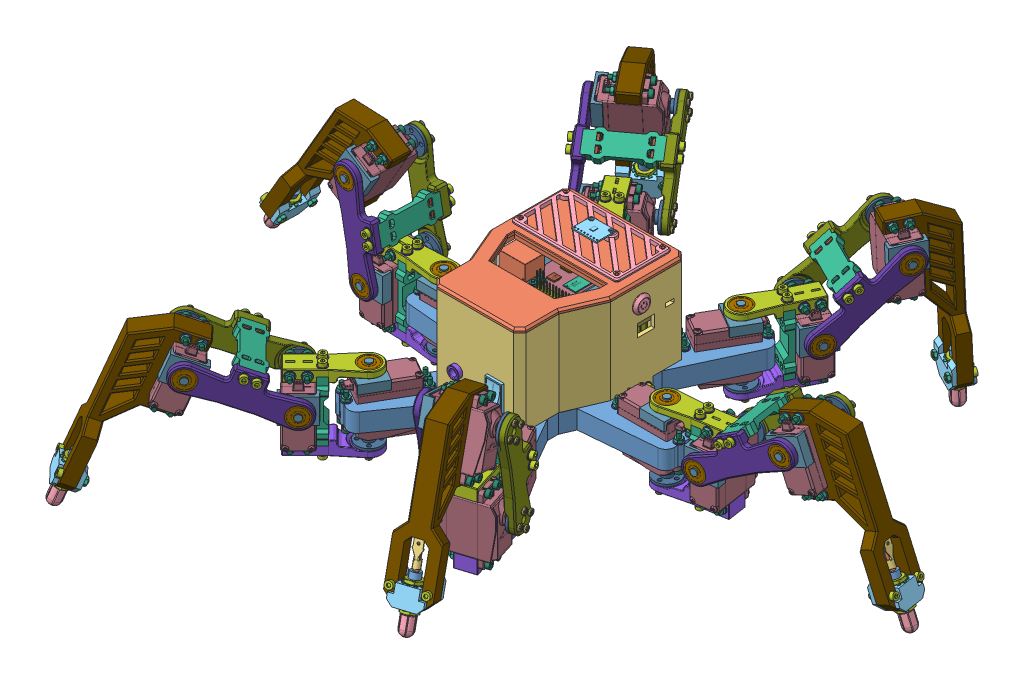
SolidWorks assembly HEXUMI_DSSERVO, configuration Default. Lengths in mm. (continued)
Components (placement in the parent): (continued)
- LEG_R-2: LEG_R [Default] at (64.2974 -8.25 149.3441) x (0.953158 0 -0.302473) z (-0.302473 0 -0.953158) size (67.5 178.11 186.84) (flexible) (continued)
  - M3_WASHER-11: M3_WASHER [Default] at (32.5 -42.9736 -1.217) x (0 0.946468 0.322799) z (0 0.322799 -0.946468) size (7 0.5 7)
  - M3_WASHER-12: M3_WASHER [Default] at (32.5 -50.8556 -2.5855) x (0 0.864489 0.502652) z (0 0.502652 -0.864489) size (7 0.5 7)
  - M3_SQUARE_NUT-10: M3_SQUARE_NUT [Default] at (-14.7 -42.9736 -1.217) x (0 -0.985259 -0.171071) z (0 -0.171071 0.985259) size (5.3 1.7 5.3)
  - M3_SQUARE_NUT-11: M3_SQUARE_NUT [Default] at (-14.7 -50.8556 -2.5855) x (0 -0.985259 -0.171071) z (0 -0.171071 0.985259) size (5.3 1.7 5.3)
  - M3_SQUARE_NUT-12: M3_SQUARE_NUT [Default] at (17.5 -42.9736 -1.217) x (0 -0.985259 -0.171071) z (0 -0.171071 0.985259) size (5.3 1.7 5.3)
  - SERVO_ASM-3: SERVO_ASM [Default] at (25.8 -78.9181 -22.175) x (0 0.943081 -0.332564) z (1 0 0) size (87.25 24.4 54.8)
    - SW2020 DS3225MG Servo 25Kg 4.8-6.8V-2: SW2020 DS3225MG Servo 25Kg 4.8-6.8V [Default] at origin size (54.3 20.4 45.91)
    - SERVO_CLIP-1: SERVO_CLIP [Default] at (0 0 -45.6) x (-1 0 0) z (0 0 -1) size (20 24.4 14.2)
  - M3_STEEL_HEX_BOLT-6: M3_STEEL_HEX_BOLT [Default] at (14.2 -94.7271 -21.9019) x (0 -0.45302 0.8915) z (0 -0.8915 -0.45302) size (5.68 28 5.68)
  - M3_STEEL_HEX_BOLT-7: M3_STEEL_HEX_BOLT [Default] at (14.2 -47.9503 -38.3971) x (0 -0.45302 0.8915) z (0 -0.8915 -0.45302) size (5.68 28 5.68)
  - M3_STEEL_HEX_BOLT-8: M3_STEEL_HEX_BOLT [Default] at (14.2 -44.6247 -28.9663) x (0 -0.45302 0.8915) z (0 -0.8915 -0.45302) size (5.68 28 5.68)
  - M3_WASHER-13: M3_WASHER [Default] at (-8.5 -91.4015 -12.4711) x (0 -0.999996 0.002865) z (0 0.002865 0.999996) size (7 0.5 7)
  - M3_WASHER-14: M3_WASHER [Default] at (-8.5 -47.9503 -38.3971) x (0 -0.195932 -0.980617) z (0 -0.980617 0.195932) size (7 0.5 7)
  - M3_WASHER-15: M3_WASHER [Default] at (-8.5 -94.7271 -21.9019) x (0 -0.288509 0.957477) z (0 0.957477 0.288509) size (7 0.5 7)
  - M3_HEX_NUT-9: M3_HEX_NUT [Default] at (-8.5 -91.4015 -12.4711) x (0 -1 -0.0006) z (0 0.0006 -1) size (6.98 2.4 5.5)
  - M3_HEX_NUT-10: M3_HEX_NUT [Default] at (-8.5 -94.7271 -21.9019) x (0 -0.879232 0.476394) z (0 -0.476394 -0.879232) size (6.98 2.4 5.5)
  - M3_HEX_NUT-11: M3_HEX_NUT [Default] at (-8.5 -44.6247 -28.9663) x (0 -0.979734 0.200301) z (0 -0.200301 -0.979734) size (6.98 2.4 5.5)
  - M3_WASHER-17: M3_WASHER [Default] at (-8.5 -44.6247 -28.9663) x (0 -0.482932 0.875658) z (0 0.875658 0.482932) size (7 0.5 7)
  - M3_SERVO_HORN_BOLT-15: M3_SERVO_HORN_BOLT [Default] at (0 28.25 30) x (0.155386 0 -0.987854) z (-0.987854 0 -0.155386) size (4.8 7 4.8)
  - M3_HEX_NUT-12: M3_HEX_NUT [Default] at (-10.9 -24.75 -5.2) x (0 -0.133559 0.991041) z (0 0.991041 0.133559) size (6.98 2.4 5.5)
  - M3_STEEL_HEX_BOLT-9: M3_STEEL_HEX_BOLT [Default] at (14.2 -24.75 -5.2) x (0 -0.73374 -0.679431) z (0 0.679431 -0.73374) size (5.68 28 5.68)
  - M3_WASHER-18: M3_WASHER [Default] at (-8.5 -24.75 -5.2) x (0 -0.999705 0.024279) z (0 0.024279 0.999705) size (7 0.5 7)
  - M3_STEEL_HEX_BOLT-10: M3_STEEL_HEX_BOLT [Default] at (14.2 -24.75 -15.2) x (0 -0.740024 -0.67258) z (0 0.67258 -0.740024) size (5.68 28 5.68)
  - M3_STEEL_HEX_BOLT-11: M3_STEEL_HEX_BOLT [Default] at (14.2 24.85 -5.2) x (0 -0.741809 -0.670611) z (0 0.670611 -0.741809) size (5.68 28 5.68)
  - M3_STEEL_HEX_BOLT-12: M3_STEEL_HEX_BOLT [Default] at (14.2 24.85 -15.2) x (0 0.582747 -0.812654) z (0 0.812654 0.582747) size (5.68 28 5.68)
  - M3_HEX_NUT-13: M3_HEX_NUT [Default] at (-10.9 24.85 -15.2) x (0 0.525669 0.850689) z (0 0.850689 -0.525669) size (6.98 2.4 5.5)
  - M3_WASHER-19: M3_WASHER [Default] at (-8.5 24.85 -15.2) x (0 -0.601111 0.799166) z (0 0.799166 0.601111) size (7 0.5 7)
  - M3_HEX_NUT-14: M3_HEX_NUT [Default] at (-10.9 24.85 -5.2) x (0 -0.636716 -0.771098) z (0 -0.771098 0.636716) size (6.98 2.4 5.5)
  - M3_WASHER-20: M3_WASHER [Default] at (-8.5 24.85 -5.2) x (0 -0.786332 -0.617804) z (0 -0.617804 0.786332) size (7 0.5 7)
  - M3_HEX_NUT-15: M3_HEX_NUT [Default] at (-10.9 -24.75 -15.2) x (0 0.444007 -0.896023) z (0 -0.896023 -0.444007) size (6.98 2.4 5.5)
  - M3_WASHER-21: M3_WASHER [Default] at (-8.5 -24.75 -15.2) x (0 -0.943365 -0.331756) z (0 -0.331756 0.943365) size (7 0.5 7)
  - TIBIA_V2_ASM-1: TIBIA_V2_ASM [Default] at (0 -78.9958 -22.0946) x (-1 0 0) z (0 -0.943081 0.332564) size (32.11 50.6 145.7)
    - TIBIA_V2-1: TIBIA_V2 [Default] at origin size (32 47.6 127.94)
    - LIMIT_SWITCH-1: LIMIT_SWITCH [Default] at (0 32.3524 -111.7407) x (-0.992713 0.1205 0) z (0.1205 0.992713 0) size (13.8 62.3 13.8) (flexible)
      - LIMIT_SWITCH_SLEEVE-1: LIMIT_SWITCH_SLEEVE [Default] at origin size (7.7 25.25 7.7)
      - LIMIT_SWITCH_SHAFT-1: LIMIT_SWITCH_SHAFT [Default] at (0 5.5422 0) x (-0.210419 0 -0.977611) z (0.977611 0 -0.210419) size (5 52 5)
      - LIMIT_SWITCH_LIMITER-1: LIMIT_SWITCH_LIMITER [Default] at (0 26.0422 0) x (-0.600712 0 -0.799465) z (0.799465 0 -0.600712) size (6.64 21.41 7.08)
      - RUBBER_CAP-1: RUBBER_CAP [Default] at (0 -9.9578 0) x (0.575853 0 -0.817553) z (0.817553 0 0.575853) size (10 14 10)
    - FOOT_HOLD-1: FOOT_HOLD [Default] at (0 32.3524 -108.9407) x (1 0 0) z (0 -1 0) size (32 22 16)
    - LIMIT_SWITCH_WASHER-1: LIMIT_SWITCH_WASHER [Default] at (0 32.3524 -93.5407) x (0.999093 -0.042592 0) z (0.042592 0.999093 0) size (14.82 0.4 15)
    - LIMIT_SWITCH_WASHER-2: LIMIT_SWITCH_WASHER [Default] at (0 32.3524 -108.9407) x (0.999093 -0.042592 0) z (0.042592 0.999093 0) size (14.82 0.4 15)
    - LIMIT_SWITCH_NUT-1: LIMIT_SWITCH_NUT [Default] at (0 32.3524 -92.3407) x (0.997292 -0.073548 0) z (0.073548 0.997292 0) size (13.86 2.4 12)
    - LIMIT_SWITCH_NUT-2: LIMIT_SWITCH_NUT [Default] at (0 32.3524 -110.5407) x (0.999648 -0.026514 0) z (0.026514 0.999648 0) size (13.86 2.4 12)
    - M3_HEX_NUT-1: M3_HEX_NUT [Default] at (-12 21.9524 -96.9407) x (-0.996596 0 -0.082443) z (0.082443 0 -0.996596) size (6.98 2.4 5.5)
    - M3_HEX_NUT-2: M3_HEX_NUT [Default] at (12 21.9524 -96.9407) x (-0.491735 0 -0.870745) z (0.870745 0 -0.491735) size (6.98 2.4 5.5)
    - M3_STEEL_HEX_BOLT_16MM-1: M3_STEEL_HEX_BOLT_16MM [Default] at (-12 40.3524 -96.9407) x (-0.809803 0 -0.586702) z (-0.586702 0 0.809803) size (5.68 19 5.68)
    - M3_STEEL_HEX_BOLT_16MM-2: M3_STEEL_HEX_BOLT_16MM [Default] at (12 40.3524 -96.9407) x (-0.933551 0 -0.358443) z (-0.358443 0 0.933551) size (5.68 19 5.68)
- LEG_R-3: LEG_R [Default] at (68.2717 -8.25 -96.793) x (-0.894785 0 -0.446496) z (-0.446496 0 0.894785) size (67.5 178.11 186.84) (flexible)
  - LINK-1: LINK [Default] at origin size (20 48.5 7)
  - COXA_BEARING-1: COXA_BEARING [Default] at (0 -29.25 30) size (20 9.2 60)
  - COXA_SERVO-1: COXA_SERVO [Default] at (0 31.25 30) x (-1 0 0) z (0 0 1) size (20 11.2 60)
  - BEARING-1: BEARING [Default] at (0 -24.25 30) x (0.102919 0 0.99469) z (0 -1 0) size (16 16 5)
  - HORN-1: HORN [Default] at (0 26.25 30) x (0 0 -1) z (0 -1 0) size (20 20 4.6)
  - M3_SQUARE_NUT-1: M3_SQUARE_NUT [Default] at (-4 16.25 3.5) x (0.944757 0 -0.327772) z (0.327772 0 0.944757) size (5.3 1.7 5.3)
  - M3_STEEL_HEX_BOLT_16MM-1: M3_STEEL_HEX_BOLT_16MM [Default] at (4 34.75 3.5) x (-0.875719 0 0.482821) z (0.482821 0 0.875719) size (5.68 19 5.68)
  - M3_WASHER-1: M3_WASHER [Default] at (4 31.25 3.5) x (0.984161 0 0.177277) z (-0.177277 0 0.984161) size (7 0.5 7)
  - M3_SERVO_HORN_BOLT-1: M3_SERVO_HORN_BOLT [Default] at (-7 33.25 30) x (-0.808099 0 -0.589047) z (-0.589047 0 0.808099) size (4.8 7 4.8)
  - M3_SERVO_HORN_BOLT-2: M3_SERVO_HORN_BOLT [Default] at (7 33.25 30) x (-0.808099 0 -0.589047) z (-0.589047 0 0.808099) size (4.8 7 4.8)
  - M3_SERVO_HORN_BOLT-3: M3_SERVO_HORN_BOLT [Default] at (0 33.25 37) x (-0.808099 0 -0.589047) z (-0.589047 0 0.808099) size (4.8 7 4.8)
  - M3_SERVO_HORN_BOLT-4: M3_SERVO_HORN_BOLT [Default] at (0 33.25 23) x (-0.808099 0 -0.589047) z (-0.589047 0 0.808099) size (4.8 7 4.8)
  - M3_SQUARE_NUT-2: M3_SQUARE_NUT [Default] at (4 16.25 3.5) x (0.947931 0 -0.318475) z (0.318475 0 0.947931) size (5.3 1.7 5.3)
  - M3_SQUARE_NUT-3: M3_SQUARE_NUT [Default] at (-4 -15.95 3.5) x (0.944757 0 -0.327772) z (0.327772 0 0.944757) size (5.3 1.7 5.3)
  - M3_SQUARE_NUT-4: M3_SQUARE_NUT [Default] at (4 -15.95 3.5) x (0.944757 0 -0.327772) z (0.327772 0 0.944757) size (5.3 1.7 5.3)
  - M3_STEEL_HEX_BOLT_16MM-2: M3_STEEL_HEX_BOLT_16MM [Default] at (-4 -32.75 3.5) x (0.944757 0 -0.327772) z (0.327772 0 0.944757) size (5.68 19 5.68)
  - M3_STEEL_HEX_BOLT_16MM-3: M3_STEEL_HEX_BOLT_16MM [Default] at (4 -32.75 3.5) x (0.944757 0 -0.327772) z (0.327772 0 0.944757) size (5.68 19 5.68)
  - M3_STEEL_HEX_BOLT_16MM-4: M3_STEEL_HEX_BOLT_16MM [Default] at (-4 34.75 3.5) x (-0.748645 0 0.662971) z (0.662971 0 0.748645) size (5.68 19 5.68)
  - M3_WASHER-2: M3_WASHER [Default] at (4 -29.75 3.5) x (0.938378 0 -0.34561) z (0.34561 0 0.938378) size (7 0.5 7)
  - M3_WASHER-3: M3_WASHER [Default] at (-4 -29.75 3.5) x (0.835901 0 -0.54888) z (0.54888 0 0.835901) size (7 0.5 7)
  - M3_WASHER-4: M3_WASHER [Default] at (-4 31.25 3.5) x (0.997383 0 -0.072301) z (0.072301 0 0.997383) size (7 0.5 7)
  - SERVO_ASM-1: SERVO_ASM [Default] at (25.8 -9.95 -10.2) x (0 1 0) z (1 0 0) size (87.25 24.4 54.8)
    - SW2020 DS3225MG Servo 25Kg 4.8-6.8V-2: SW2020 DS3225MG Servo 25Kg 4.8-6.8V [Default] at origin size (54.3 20.4 45.91)
    - SERVO_CLIP-1: SERVO_CLIP [Default] at (0 0 -45.6) x (-1 0 0) z (0 0 -1) size (20 24.4 14.2)
  - SERVO_ASM-2: SERVO_ASM [Default] at (0 24.55 30) x (0.060715 0 0.998155) z (0 1 0) size (87.25 24.4 54.8)
    - SW2020 DS3225MG Servo 25Kg 4.8-6.8V-2: SW2020 DS3225MG Servo 25Kg 4.8-6.8V [Default] at origin size (54.3 20.4 45.91)
    - SERVO_CLIP-1: SERVO_CLIP [Default] at (0 0 -45.6) x (-1 0 0) z (0 0 -1) size (20 24.4 14.2)
  - M3_SQUARE_NUT-5: M3_SQUARE_NUT [Default] at (0.85 24.85 -15.2) x (0 0 -1) z (0 1 0) size (5.3 1.7 5.3)
  - M3_SQUARE_NUT-6: M3_SQUARE_NUT [Default] at (0.85 -24.75 -5.2) x (0 1 0) z (0 0 1) size (5.3 1.7 5.3)
  - M3_SQUARE_NUT-7: M3_SQUARE_NUT [Default] at (0.85 -24.75 -15.2) x (0 1 0) z (0 0 1) size (5.3 1.7 5.3)
  - M3_SQUARE_NUT-8: M3_SQUARE_NUT [Default] at (0.85 24.85 -5.2) x (0 0 -1) z (0 1 0) size (5.3 1.7 5.3)
  - FEMUR_SERVO-1: FEMUR_SERVO [Default] at (32.5 -9.95 -10.2) x (-1 0 0) z (0 0.640618 0.76786) size (10 28 90)
  - FEMUR_BEARING-1: FEMUR_BEARING [Default] at (-28 -54.7933 -63.9502) x (1 0 0) z (0 -0.640618 -0.76786) size (8 28 90)
  - LINK-2: LINK [Default] at (1.25 -46.1931 -25.544) x (0 0.640618 0.76786) z (0 0.76786 -0.640618) size (20 48.5 7)
  - BEARING-2: BEARING [Default] at (-28 -54.7933 -63.9502) x (0 0.859543 0.511064) z (1 0 0) size (16 16 5)
  - HORN-2: HORN [Default] at (27.5 -54.7933 -63.9502) x (0 -0.76786 0.640618) z (-1 0 0) size (20 20 4.6)
  - BEARING-3: BEARING [Default] at (-28 -9.95 -10.2) x (0 0.859543 0.511064) z (1 0 0) size (16 16 5)
  - HORN-3: HORN [Default] at (27.5 -9.95 -10.2) x (0 -0.640618 -0.76786) z (-1 0 0) size (20 20 4.6)
  - M3_HEX_NUT-5: M3_HEX_NUT [Default] at (-8.5 -20.4015 -70.2245) x (0 -0.795634 0.605778) z (0 -0.605778 -0.795634) size (6.98 2.4 5.5)
  - M3_SERVO_HORN_BOLT-5: M3_SERVO_HORN_BOLT [Default] at (34.5 -60.1683 -59.4658) x (0 -0.164589 0.986362) z (0 -0.986362 -0.164589) size (4.8 7 4.8)
  - M3_SQUARE_NUT-9: M3_SQUARE_NUT [Default] at (17.5 -46.0681 -30.8576) x (0 -0.640618 -0.76786) z (0 -0.76786 0.640618) size (5.3 1.7 5.3)
  - M3_STEEL_HEX_BOLT-5: M3_STEEL_HEX_BOLT [Default] at (14.2 -69.5984 -58.3997) x (0 -0.45302 0.8915) z (0 -0.8915 -0.45302) size (5.68 28 5.68)
  - M3_STEEL_HEX_BOLT_16MM-5: M3_STEEL_HEX_BOLT_16MM [Default] at (-31.5 -46.0681 -30.8576) x (0 0.164045 0.986453) z (0 0.986453 -0.164045) size (5.68 19 5.68)
  - M3_WASHER-9: M3_WASHER [Default] at (-28.5 -46.0681 -30.8576) x (0 0.889965 0.456029) z (0 0.456029 -0.889965) size (7 0.5 7)
  - M3_SERVO_HORN_BOLT-6: M3_SERVO_HORN_BOLT [Default] at (34.5 -49.4183 -68.4345) x (0 -0.961641 0.27431) z (0 -0.27431 -0.961641) size (4.8 7 4.8)
  - M3_SERVO_HORN_BOLT-7: M3_SERVO_HORN_BOLT [Default] at (34.5 -14.4343 -15.575) x (0 -0.974393 0.224852) z (0 -0.224852 -0.974393) size (4.8 7 4.8)
  - M3_SERVO_HORN_BOLT-8: M3_SERVO_HORN_BOLT [Default] at (34.5 -4.575 -14.6843) x (0 -0.996733 0.080764) z (0 -0.080764 -0.996733) size (4.8 7 4.8)
  - M3_SERVO_HORN_BOLT-9: M3_SERVO_HORN_BOLT [Default] at (34.5 -15.325 -5.7157) x (0 -0.79921 0.601052) z (0 -0.601052 -0.79921) size (4.8 7 4.8)
  - M3_SERVO_HORN_BOLT-10: M3_SERVO_HORN_BOLT [Default] at (34.5 -5.4657 -4.825) x (0 -0.903711 0.428143) z (0 -0.428143 -0.903711) size (4.8 7 4.8)
  - M3_SERVO_HORN_BOLT-11: M3_SERVO_HORN_BOLT [Default] at (34.5 -59.2776 -69.3252) x (0 -0.961939 -0.273266) z (0 0.273266 -0.961939) size (4.8 7 4.8)
  - M3_SERVO_HORN_BOLT-12: M3_SERVO_HORN_BOLT [Default] at (34.5 -50.3089 -58.5752) x (0 -0.806511 0.591219) z (0 -0.591219 -0.806511) size (4.8 7 4.8)
  - M3_SERVO_HORN_BOLT-13: M3_SERVO_HORN_BOLT [Default] at (29.5 -9.95 -10.2) x (0 -0.903711 0.428143) z (0 -0.428143 -0.903711) size (4.8 7 4.8)
  - M3_SERVO_HORN_BOLT-14: M3_SERVO_HORN_BOLT [Default] at (29.5 -54.7933 -63.9502) x (0 -0.903711 0.428143) z (0 -0.428143 -0.903711) size (4.8 7 4.8)
  - M3_STEEL_HEX_BOLT_16MM-6: M3_STEEL_HEX_BOLT_16MM [Default] at (36 -40.9431 -24.7147) x (0 -0.934703 -0.35543) z (0 0.35543 -0.934703) size (5.68 19 5.68)
  - M3_STEEL_HEX_BOLT_16MM-7: M3_STEEL_HEX_BOLT_16MM [Default] at (-31.5 -40.9431 -24.7147) x (0 0.433334 0.901233) z (0 0.901233 -0.433334) size (5.68 19 5.68)
  - M3_STEEL_HEX_BOLT_16MM-8: M3_STEEL_HEX_BOLT_16MM [Default] at (36 -46.0681 -30.8576) x (0 -0.762342 -0.647175) z (0 0.647175 -0.762342) size (5.68 19 5.68)
  - M3_WASHER-10: M3_WASHER [Default] at (-28.5 -40.9431 -24.7147) x (0 0.908707 0.417435) z (0 0.417435 -0.908707) size (7 0.5 7)
  - M3_WASHER-11: M3_WASHER [Default] at (32.5 -40.9431 -24.7147) x (0 0.946468 0.322799) z (0 0.322799 -0.946468) size (7 0.5 7)
  - M3_WASHER-12: M3_WASHER [Default] at (32.5 -46.0681 -30.8576) x (0 0.864489 0.502652) z (0 0.502652 -0.864489) size (7 0.5 7)
  - M3_SQUARE_NUT-10: M3_SQUARE_NUT [Default] at (-14.7 -40.9431 -24.7147) x (0 -0.640618 -0.76786) z (0 -0.76786 0.640618) size (5.3 1.7 5.3)
  - M3_SQUARE_NUT-11: M3_SQUARE_NUT [Default] at (-14.7 -46.0681 -30.8576) x (0 -0.640618 -0.76786) z (0 -0.76786 0.640618) size (5.3 1.7 5.3)
  - M3_SQUARE_NUT-12: M3_SQUARE_NUT [Default] at (17.5 -40.9431 -24.7147) x (0 -0.640618 -0.76786) z (0 -0.76786 0.640618) size (5.3 1.7 5.3)
  - SERVO_ASM-3: SERVO_ASM [Default] at (25.8 -54.7933 -63.9502) x (0 0.999318 -0.036928) z (1 0 0) size (87.25 24.4 54.8)
    - SW2020 DS3225MG Servo 25Kg 4.8-6.8V-2: SW2020 DS3225MG Servo 25Kg 4.8-6.8V [Default] at origin size (54.3 20.4 45.91)
    - SERVO_CLIP-1: SERVO_CLIP [Default] at (0 0 -45.6) x (-1 0 0) z (0 0 -1) size (20 24.4 14.2)
  - M3_STEEL_HEX_BOLT-6: M3_STEEL_HEX_BOLT [Default] at (14.2 -69.9677 -68.3928) x (0 -0.45302 0.8915) z (0 -0.8915 -0.45302) size (5.68 28 5.68)
  - M3_STEEL_HEX_BOLT-7: M3_STEEL_HEX_BOLT [Default] at (14.2 -20.4015 -70.2245) x (0 -0.45302 0.8915) z (0 -0.8915 -0.45302) size (5.68 28 5.68)
  - M3_STEEL_HEX_BOLT-8: M3_STEEL_HEX_BOLT [Default] at (14.2 -20.0322 -60.2313) x (0 -0.45302 0.8915) z (0 -0.8915 -0.45302) size (5.68 28 5.68)
  - M3_WASHER-13: M3_WASHER [Default] at (-8.5 -69.5984 -58.3997) x (0 -0.999996 0.002865) z (0 0.002865 0.999996) size (7 0.5 7)
  - M3_WASHER-14: M3_WASHER [Default] at (-8.5 -20.4015 -70.2245) x (0 -0.195932 -0.980617) z (0 -0.980617 0.195932) size (7 0.5 7)
  - M3_WASHER-15: M3_WASHER [Default] at (-8.5 -69.9677 -68.3928) x (0 -0.288509 0.957477) z (0 0.957477 0.288509) size (7 0.5 7)
  - M3_HEX_NUT-9: M3_HEX_NUT [Default] at (-8.5 -69.5984 -58.3997) x (0 -1 -0.0006) z (0 0.0006 -1) size (6.98 2.4 5.5)
  - M3_HEX_NUT-10: M3_HEX_NUT [Default] at (-8.5 -69.9677 -68.3928) x (0 -0.879232 0.476394) z (0 -0.476394 -0.879232) size (6.98 2.4 5.5)
  - M3_HEX_NUT-11: M3_HEX_NUT [Default] at (-8.5 -20.0322 -60.2313) x (0 -0.979734 0.200301) z (0 -0.200301 -0.979734) size (6.98 2.4 5.5)
  - M3_WASHER-17: M3_WASHER [Default] at (-8.5 -20.0322 -60.2313) x (0 -0.482932 0.875658) z (0 0.875658 0.482932) size (7 0.5 7)
  - M3_SERVO_HORN_BOLT-15: M3_SERVO_HORN_BOLT [Default] at (0 28.25 30) x (-0.120751 0 -0.992683) z (-0.992683 0 0.120751) size (4.8 7 4.8)
  - M3_HEX_NUT-12: M3_HEX_NUT [Default] at (-10.9 -24.75 -5.2) x (0 -0.133559 0.991041) z (0 0.991041 0.133559) size (6.98 2.4 5.5)
  - M3_STEEL_HEX_BOLT-9: M3_STEEL_HEX_BOLT [Default] at (14.2 -24.75 -5.2) x (0 -0.73374 -0.679431) z (0 0.679431 -0.73374) size (5.68 28 5.68)
  - M3_WASHER-18: M3_WASHER [Default] at (-8.5 -24.75 -5.2) x (0 -0.999705 0.024279) z (0 0.024279 0.999705) size (7 0.5 7)
  - M3_STEEL_HEX_BOLT-10: M3_STEEL_HEX_BOLT [Default] at (14.2 -24.75 -15.2) x (0 -0.740024 -0.67258) z (0 0.67258 -0.740024) size (5.68 28 5.68)
  - M3_STEEL_HEX_BOLT-11: M3_STEEL_HEX_BOLT [Default] at (14.2 24.85 -5.2) x (0 -0.741809 -0.670611) z (0 0.670611 -0.741809) size (5.68 28 5.68)
  - M3_STEEL_HEX_BOLT-12: M3_STEEL_HEX_BOLT [Default] at (14.2 24.85 -15.2) x (0 0.582747 -0.812654) z (0 0.812654 0.582747) size (5.68 28 5.68)
  - M3_HEX_NUT-13: M3_HEX_NUT [Default] at (-10.9 24.85 -15.2) x (0 0.525669 0.850689) z (0 0.850689 -0.525669) size (6.98 2.4 5.5)
  - M3_WASHER-19: M3_WASHER [Default] at (-8.5 24.85 -15.2) x (0 -0.601111 0.799166) z (0 0.799166 0.601111) size (7 0.5 7)
  - M3_HEX_NUT-14: M3_HEX_NUT [Default] at (-10.9 24.85 -5.2) x (0 -0.636716 -0.771098) z (0 -0.771098 0.636716) size (6.98 2.4 5.5)
  - M3_WASHER-20: M3_WASHER [Default] at (-8.5 24.85 -5.2) x (0 -0.786332 -0.617804) z (0 -0.617804 0.786332) size (7 0.5 7)
  - M3_HEX_NUT-15: M3_HEX_NUT [Default] at (-10.9 -24.75 -15.2) x (0 0.444007 -0.896023) z (0 -0.896023 -0.444007) size (6.98 2.4 5.5)
  - M3_WASHER-21: M3_WASHER [Default] at (-8.5 -24.75 -15.2) x (0 -0.943365 -0.331756) z (0 -0.331756 0.943365) size (7 0.5 7)
  - TIBIA_V2_ASM-1: TIBIA_V2_ASM [Default] at (0 -54.8914 -63.8965) x (-1 0 0) z (0 -0.999318 0.036928) size (32.11 50.6 145.7)
    - TIBIA_V2-1: TIBIA_V2 [Default] at origin size (32 47.6 127.94)
    - LIMIT_SWITCH-1: LIMIT_SWITCH [Default] at (0 32.3524 -111.7407) x (-0.992713 0.1205 0) z (0.1205 0.992713 0) size (13.8 62.3 13.8) (flexible)
      - LIMIT_SWITCH_SLEEVE-1: LIMIT_SWITCH_SLEEVE [Default] at origin size (7.7 25.25 7.7)
      - LIMIT_SWITCH_SHAFT-1: LIMIT_SWITCH_SHAFT [Default] at (0 5.5422 0) x (-0.210419 0 -0.977611) z (0.977611 0 -0.210419) size (5 52 5)
      - LIMIT_SWITCH_LIMITER-1: LIMIT_SWITCH_LIMITER [Default] at (0 26.0422 0) x (-0.600712 0 -0.799465) z (0.799465 0 -0.600712) size (6.64 21.41 7.08)
      - RUBBER_CAP-1: RUBBER_CAP [Default] at (0 -9.9578 0) x (0.575853 0 -0.817553) z (0.817553 0 0.575853) size (10 14 10)
    - FOOT_HOLD-1: FOOT_HOLD [Default] at (0 32.3524 -108.9407) x (1 0 0) z (0 -1 0) size (32 22 16)
    - LIMIT_SWITCH_WASHER-1: LIMIT_SWITCH_WASHER [Default] at (0 32.3524 -93.5407) x (0.999093 -0.042592 0) z (0.042592 0.999093 0) size (14.82 0.4 15)
    - LIMIT_SWITCH_WASHER-2: LIMIT_SWITCH_WASHER [Default] at (0 32.3524 -108.9407) x (0.999093 -0.042592 0) z (0.042592 0.999093 0) size (14.82 0.4 15)
    - LIMIT_SWITCH_NUT-1: LIMIT_SWITCH_NUT [Default] at (0 32.3524 -92.3407) x (0.997292 -0.073548 0) z (0.073548 0.997292 0) size (13.86 2.4 12)
    - LIMIT_SWITCH_NUT-2: LIMIT_SWITCH_NUT [Default] at (0 32.3524 -110.5407) x (0.999648 -0.026514 0) z (0.026514 0.999648 0) size (13.86 2.4 12)
    - M3_HEX_NUT-1: M3_HEX_NUT [Default] at (-12 21.9524 -96.9407) x (-0.996596 0 -0.082443) z (0.082443 0 -0.996596) size (6.98 2.4 5.5)
    - M3_HEX_NUT-2: M3_HEX_NUT [Default] at (12 21.9524 -96.9407) x (-0.491735 0 -0.870745) z (0.870745 0 -0.491735) size (6.98 2.4 5.5)
    - M3_STEEL_HEX_BOLT_16MM-1: M3_STEEL_HEX_BOLT_16MM [Default] at (-12 40.3524 -96.9407) x (-0.809803 0 -0.586702) z (-0.586702 0 0.809803) size (5.68 19 5.68)
    - M3_STEEL_HEX_BOLT_16MM-2: M3_STEEL_HEX_BOLT_16MM [Default] at (12 40.3524 -96.9407) x (-0.933551 0 -0.358443) z (-0.358443 0 0.933551) size (5.68 19 5.68)
- M3_STEEL_HEX_BOLT-1: M3_STEEL_HEX_BOLT [Default] at (66.9533 -21.2 131.0666) size (5.68 28 5.68)
- M3_WASHER-1: M3_WASHER [Default] at (-58.2931 0 136.0666) size (7 0.5 7)
- M3_STEEL_HEX_BOLT-2: M3_STEEL_HEX_BOLT [Default] at (104.9 -21.2 30.3) size (5.68 28 5.68)
- M3_STEEL_HEX_BOLT-3: M3_STEEL_HEX_BOLT [Default] at (-58.2931 -21.2 136.0666) size (5.68 28 5.68)
- M3_STEEL_HEX_BOLT-4: M3_STEEL_HEX_BOLT [Default] at (-41.8069 -21.2 -37.3117) x (0.933508 0 -0.358556) z (0.358556 0 0.933508) size (5.68 28 5.68)
- M3_STEEL_HEX_BOLT-5: M3_STEEL_HEX_BOLT [Default] at (41.8069 -21.2 -37.3117) size (5.68 28 5.68)
- M3_STEEL_HEX_BOLT-6: M3_STEEL_HEX_BOLT [Default] at (55.3 -21.2 20.3) size (5.68 28 5.68)
- M3_STEEL_HEX_BOLT-7: M3_STEEL_HEX_BOLT [Default] at (55.3 -21.2 30.3) size (5.68 28 5.68)
- M3_STEEL_HEX_BOLT-8: M3_STEEL_HEX_BOLT [Default] at (42.1533 -21.2 88.1117) size (5.68 28 5.68)
- M3_STEEL_HEX_BOLT-9: M3_STEEL_HEX_BOLT [Default] at (33.4931 -21.2 93.1117) x (-0.097686 0 -0.995217) z (0.995217 0 -0.097686) size (5.68 28 5.68)
- M3_STEEL_HEX_BOLT-10: M3_STEEL_HEX_BOLT [Default] at (-55.3 -21.2 20.3) size (5.68 28 5.68)
- M3_STEEL_HEX_BOLT-11: M3_STEEL_HEX_BOLT [Default] at (-55.3 -21.2 30.3) size (5.68 28 5.68)
- M3_STEEL_HEX_BOLT-12: M3_STEEL_HEX_BOLT [Default] at (-33.4931 -21.2 93.1117) size (5.68 28 5.68)
- M3_STEEL_HEX_BOLT-13: M3_STEEL_HEX_BOLT [Default] at (-42.1533 -21.2 88.1117) x (0.960294 0 -0.278991) z (0.278991 0 0.960294) size (5.68 28 5.68)
- M3_STEEL_HEX_BOLT-14: M3_STEEL_HEX_BOLT [Default] at (104.9 -21.2 20.3) size (5.68 28 5.68)
- M3_STEEL_HEX_BOLT-15: M3_STEEL_HEX_BOLT [Default] at (66.6069 -21.2 -80.2666) size (5.68 28 5.68)
- M3_STEEL_HEX_BOLT-16: M3_STEEL_HEX_BOLT [Default] at (57.9467 -21.2 -85.2666) size (5.68 28 5.68)
- M3_STEEL_HEX_BOLT-17: M3_STEEL_HEX_BOLT [Default] at (-66.6069 -21.2 -80.2666) size (5.68 28 5.68)
- M3_STEEL_HEX_BOLT-18: M3_STEEL_HEX_BOLT [Default] at (-57.9467 -21.2 -85.2666) size (5.68 28 5.68)
- M3_STEEL_HEX_BOLT-19: M3_STEEL_HEX_BOLT [Default] at (-104.9 -21.2 20.3) size (5.68 28 5.68)
- M3_STEEL_HEX_BOLT-20: M3_STEEL_HEX_BOLT [Default] at (-104.9 -21.2 30.3) x (0.992945 0 -0.118579) z (0.118579 0 0.992945) size (5.68 28 5.68)
- M3_STEEL_HEX_BOLT-21: M3_STEEL_HEX_BOLT [Default] at (-66.9533 -21.2 131.0666) size (5.68 28 5.68)
- M3_STEEL_HEX_BOLT-22: M3_STEEL_HEX_BOLT [Default] at (-33.1467 -21.2 -42.3117) x (-0.575955 0 -0.817481) z (0.817481 0 -0.575955) size (5.68 28 5.68)
- M3_STEEL_HEX_BOLT-23: M3_STEEL_HEX_BOLT [Default] at (33.1467 -21.2 -42.3117) size (5.68 28 5.68)
- M3_STEEL_HEX_BOLT-24: M3_STEEL_HEX_BOLT [Default] at (58.2931 -21.2 136.0666) size (5.68 28 5.68)
- M3_WASHER-2: M3_WASHER [Default] at (42.1533 0 88.1117) x (-0.195922 0 0.980619) z (-0.980619 0 -0.195922) size (7 0.5 7)
- M3_WASHER-3: M3_WASHER [Default] at (104.9 0 30.3) size (7 0.5 7)
- M3_WASHER-4: M3_WASHER [Default] at (55.3 0 20.3) size (7 0.5 7)
- M3_WASHER-5: M3_WASHER [Default] at (41.8069 0 -37.3117) size (7 0.5 7)
- M3_WASHER-6: M3_WASHER [Default] at (-42.1533 0 88.1117) size (7 0.5 7)
- M3_WASHER-7: M3_WASHER [Default] at (55.3 0 30.3) size (7 0.5 7)
- M3_WASHER-8: M3_WASHER [Default] at (-66.9533 0 131.0666) size (7 0.5 7)
- M3_WASHER-9: M3_WASHER [Default] at (33.1467 0 -42.3117) size (7 0.5 7)
- M3_WASHER-10: M3_WASHER [Default] at (-33.4931 0 93.1117) x (-0.942 0 0.335612) z (-0.335612 0 -0.942) size (7 0.5 7)
- M3_WASHER-11: M3_WASHER [Default] at (-41.8069 0 -37.3117) size (7 0.5 7)
- M3_WASHER-12: M3_WASHER [Default] at (-57.9467 0 -85.2666) size (7 0.5 7)
- M3_WASHER-13: M3_WASHER [Default] at (-33.1467 0 -42.3117) size (7 0.5 7)
- M3_WASHER-14: M3_WASHER [Default] at (-55.3 0 30.3) size (7 0.5 7)
- M3_WASHER-15: M3_WASHER [Default] at (-55.3 0 20.3) size (7 0.5 7)
- M3_WASHER-16: M3_WASHER [Default] at (-104.9 0 30.3) size (7 0.5 7)
- M3_WASHER-17: M3_WASHER [Default] at (-66.6069 0 -80.2666) size (7 0.5 7)
- M3_WASHER-18: M3_WASHER [Default] at (104.9 0 20.3) size (7 0.5 7)
- M3_WASHER-19: M3_WASHER [Default] at (33.4931 0 93.1117) x (0.999858 0 -0.016852) z (0.016852 0 0.999858) size (7 0.5 7)
- M3_WASHER-20: M3_WASHER [Default] at (66.9533 0 131.0666) size (7 0.5 7)
- M3_WASHER-21: M3_WASHER [Default] at (58.2931 0 136.0666) x (0.083375 0 -0.996518) z (0.996518 0 0.083375) size (7 0.5 7)
- M3_WASHER-22: M3_WASHER [Default] at (57.9467 0 -85.2666) size (7 0.5 7)
- M3_WASHER-23: M3_WASHER [Default] at (66.6069 0 -80.2666) x (0.999819 0 0.019033) z (-0.019033 0 0.999819) size (7 0.5 7)
- M3_HEX_NUT-2: M3_HEX_NUT [Default] at (104.9 0.5 20.3) size (6.98 2.4 5.5)
- M3_HEX_NUT-3: M3_HEX_NUT [Default] at (33.4931 0.5 93.1117) x (0.999078 0 -0.042942) z (0.042942 0 0.999078) size (6.98 2.4 5.5)
- M3_HEX_NUT-4: M3_HEX_NUT [Default] at (58.2931 0.5 136.0666) x (-0.712528 0 -0.701644) z (0.701644 0 -0.712528) size (6.98 2.4 5.5)
- M3_HEX_NUT-5: M3_HEX_NUT [Default] at (42.1533 0.5 88.1117) x (-0.077073 0 -0.997025) z (0.997025 0 -0.077073) size (6.98 2.4 5.5)
- M3_HEX_NUT-6: M3_HEX_NUT [Default] at (104.9 0.5 30.3) size (6.98 2.4 5.5)
- M3_HEX_NUT-7: M3_HEX_NUT [Default] at (55.3 0.5 30.3) size (6.98 2.4 5.5)
- M3_HEX_NUT-8: M3_HEX_NUT [Default] at (33.1467 0.5 -42.3117) size (6.98 2.4 5.5)
- M3_HEX_NUT-9: M3_HEX_NUT [Default] at (-66.9533 0.5 131.0666) size (6.98 2.4 5.5)
- M3_HEX_NUT-10: M3_HEX_NUT [Default] at (-41.8069 0.5 -37.3117) size (6.98 2.4 5.5)
- M3_HEX_NUT-11: M3_HEX_NUT [Default] at (57.9467 0.5 -85.2666) x (0.99971 0 0.024067) z (-0.024067 0 0.99971) size (6.98 2.4 5.5)
- M3_HEX_NUT-12: M3_HEX_NUT [Default] at (-33.4931 0.5 93.1117) x (0.994322 0 -0.106411) z (0.106411 0 0.994322) size (6.98 2.4 5.5)
- M3_HEX_NUT-13: M3_HEX_NUT [Default] at (55.3 0.5 20.3) size (6.98 2.4 5.5)
- M3_HEX_NUT-14: M3_HEX_NUT [Default] at (41.8069 0.5 -37.3117) size (6.98 2.4 5.5)
- M3_HEX_NUT-15: M3_HEX_NUT [Default] at (-42.1533 0.5 88.1117) size (6.98 2.4 5.5)
- M3_HEX_NUT-16: M3_HEX_NUT [Default] at (-33.1467 0.5 -42.3117) x (0.995341 0 0.096422) z (-0.096422 0 0.995341) size (6.98 2.4 5.5)
- M3_HEX_NUT-17: M3_HEX_NUT [Default] at (66.9533 0.5 131.0666) x (0.999915 0 -0.013073) z (0.013073 0 0.999915) size (6.98 2.4 5.5)
- M3_HEX_NUT-18: M3_HEX_NUT [Default] at (66.6069 0.5 -80.2666) size (6.98 2.4 5.5)
- M3_HEX_NUT-19: M3_HEX_NUT [Default] at (-55.3 0.5 30.3) size (6.98 2.4 5.5)
- M3_HEX_NUT-20: M3_HEX_NUT [Default] at (-55.3 0.5 20.3) size (6.98 2.4 5.5)
- M3_HEX_NUT-21: M3_HEX_NUT [Default] at (-57.9467 0.5 -85.2666) size (6.98 2.4 5.5)
- M3_HEX_NUT-22: M3_HEX_NUT [Default] at (-66.6069 0.5 -80.2666) size (6.98 2.4 5.5)
- M3_HEX_NUT-23: M3_HEX_NUT [Default] at (-104.9 0.5 30.3) size (6.98 2.4 5.5)
- M3_HEX_NUT-24: M3_HEX_NUT [Default] at (-58.2931 0.5 136.0666) size (6.98 2.4 5.5)
- M3_WASHER-25: M3_WASHER [Default] at (-104.9 0.5 20.3) x (0.772354 0 0.635192) z (0.635192 0 -0.772354) size (7 0.5 7)
- M3_HEX_NUT-25: M3_HEX_NUT [Default] at (-104.9 2.9 20.3) x (-0.914132 0 0.405416) z (0.405416 0 0.914132) size (6.98 2.4 5.5)
- DC_PLUG-1: DC_PLUG [Default] at (-15 19.5 90) x (0.765379 0.643579 0) z (0.643579 -0.765379 0) size (9.6 8.84 9.6)
Mates (geometry in assembly coordinates):
- Coincident1: coordinate: unknown of BODY_ASM-1
- Coincident2: coincident anti-aligned: plane of BODY_ASM-1/MAIN_FRAME-1 through (-48.6603 -15 -38.782) normal (0.866025 0 -0.5); plane of LEG_L-1/SERVO_ASM-2/SW2020 DS3225MG Servo 25Kg 4.8-6.8V-2 through (-49.1603 50.0799 -39.6481) normal (-0.866025 0 0.5)
- Coincident3: coincident anti-aligned: plane of BODY_ASM-1/MAIN_FRAME-1 through (-48.6603 -15 -38.782) normal (-0.5 0 -0.866025); plane of LEG_L-1/SERVO_ASM-2/SW2020 DS3225MG Servo 25Kg 4.8-6.8V-2 through (-31.8594 50.0799 -48.482) normal (0.5 0 0.866025)
- Coincident4: coincident anti-aligned: plane of BODY_ASM-1/MAIN_FRAME-1 through (34 -15 55.6123) normal (0 -1 0); plane of LEG_L-1/SERVO_ASM-2/SW2020 DS3225MG Servo 25Kg 4.8-6.8V-2 through (-67.3942 -15 -73.2302) normal (0 1 0)
- Coincident5: coincident anti-aligned: plane of BODY_ASM-1/MAIN_FRAME-1 through (-60 -15 35.5) normal (0 0 -1); plane of LEG_L-3/SERVO_ASM-2/SW2020 DS3225MG Servo 25Kg 4.8-6.8V-2 through (-61 50.0799 35.5) normal (0 0 1)
- Coincident6: coincident anti-aligned: plane of BODY_ASM-1/MAIN_FRAME-1 through (-60 -15 15.5) normal (-1 0 0); plane of LEG_L-3/SERVO_ASM-2/SW2020 DS3225MG Servo 25Kg 4.8-6.8V-2 through (-60 50.0799 16.1) normal (1 0 0)
- Coincident7: coincident anti-aligned: plane of BODY_ASM-1/MAIN_FRAME-1 through (34 -15 55.6123) normal (0 -1 0); plane of LEG_L-3/SERVO_ASM-2/SW2020 DS3225MG Servo 25Kg 4.8-6.8V-2 through (-99.2 -15 34.5) normal (0 1 0)
- Coincident8: coincident anti-aligned: plane of BODY_ASM-1/MAIN_FRAME-1 through (-51.3397 -15 134.423) normal (-0.866025 0 -0.5); plane of LEG_L-2/SERVO_ASM-2/SW2020 DS3225MG Servo 25Kg 4.8-6.8V-2 through (-31.8397 50.0799 100.6481) normal (0.866025 0 0.5)
- Coincident9: coincident anti-aligned: plane of BODY_ASM-1/MAIN_FRAME-1 through (-31.3397 -15 99.782) normal (-0.5 0 0.866025); plane of LEG_L-2/SERVO_ASM-2/SW2020 DS3225MG Servo 25Kg 4.8-6.8V-2 through (-48.1406 50.0799 90.082) normal (0.5 0 -0.866025)
- Coincident10: coincident anti-aligned: plane of BODY_ASM-1/MAIN_FRAME-1 through (34 -15 55.6123) normal (0 -1 0); plane of LEG_L-2/SERVO_ASM-2/SW2020 DS3225MG Servo 25Kg 4.8-6.8V-2 through (-51.8058 -15 133.2302) normal (0 1 0)
- Coincident11: coincident anti-aligned: plane of BODY_ASM-1/MAIN_FRAME-1 through (48.6603 -15 -38.782) normal (-0.866025 0 -0.5); plane of LEG_R-3/SERVO_ASM-2/SW2020 DS3225MG Servo 25Kg 4.8-6.8V-2 through (68.2603 50.0799 -72.7302) normal (0.866025 0 0.5)
- Coincident12: coincident anti-aligned: plane of BODY_ASM-1/MAIN_FRAME-1 through (48.6603 -15 -38.782) normal (0.5 0 -0.866025); plane of LEG_R-3/SERVO_ASM-2/SW2020 DS3225MG Servo 25Kg 4.8-6.8V-2 through (47.7942 50.0799 -39.282) normal (-0.5 0 0.866025)
- Coincident13: coincident anti-aligned: plane of BODY_ASM-1/MAIN_FRAME-1 through (34 -15 55.6123) normal (0 -1 0); plane of LEG_R-3/SERVO_ASM-2/SW2020 DS3225MG Servo 25Kg 4.8-6.8V-2 through (51.4594 -15 -82.4302) normal (0 1 0)
- Coincident14: coincident anti-aligned: plane of BODY_ASM-1/MAIN_FRAME-1 through (60 -15 35.5) normal (0 0 -1); plane of LEG_R-1/SERVO_ASM-2/SW2020 DS3225MG Servo 25Kg 4.8-6.8V-2 through (99.2 50.0799 35.5) normal (0 0 1)
- Coincident15: coincident anti-aligned: plane of BODY_ASM-1/MAIN_FRAME-1 through (60 -15 15.5) normal (1 0 0); plane of LEG_R-1/SERVO_ASM-2/SW2020 DS3225MG Servo 25Kg 4.8-6.8V-2 through (60 50.0799 34.5) normal (-1 0 0)
- Coincident16: coincident anti-aligned: plane of BODY_ASM-1/MAIN_FRAME-1 through (34 -15 55.6123) normal (0 -1 0); plane of LEG_R-1/SERVO_ASM-2/SW2020 DS3225MG Servo 25Kg 4.8-6.8V-2 through (99.2 -15 16.1) normal (0 1 0)
- Coincident17: coincident anti-aligned: plane of BODY_ASM-1/MAIN_FRAME-1 through (51.3397 -15 134.423) normal (0.866025 0 -0.5); plane of LEG_R-2/SERVO_ASM-2/SW2020 DS3225MG Servo 25Kg 4.8-6.8V-2 through (50.9397 50.0799 133.7302) normal (-0.866025 0 0.5)
- Coincident18: coincident anti-aligned: plane of BODY_ASM-1/MAIN_FRAME-1 through (31.3397 -15 99.782) normal (0.5 0 0.866025); plane of LEG_R-2/SERVO_ASM-2/SW2020 DS3225MG Servo 25Kg 4.8-6.8V-2 through (32.2058 50.0799 99.282) normal (-0.5 0 -0.866025)
- Coincident19: coincident anti-aligned: plane of BODY_ASM-1/MAIN_FRAME-1 through (34 -15 55.6123) normal (0 -1 0); plane of LEG_R-2/SERVO_ASM-2/SW2020 DS3225MG Servo 25Kg 4.8-6.8V-2 through (67.7406 -15 124.0302) normal (0 1 0)
- Concentric2: concentric aligned: cylinder of M3_WASHER-1 through (-58.2931 0.5 136.0666) axis (0 -1 0) radius 1.6; cylinder of M3_HEX_NUT-24 through (-58.2931 2.9 136.0666) axis (0 -1 0) radius 1.5
- Concentric4: concentric aligned: cylinder of M3_WASHER-18 through (104.9 0.5 20.3) axis (0 -1 0) radius 1.6; cylinder of M3_HEX_NUT-2 through (104.9 2.9 20.3) axis (0 -1 0) radius 1.5
- Concentric5: concentric aligned: cylinder of M3_WASHER-19 through (33.4931 0.5 93.1117) axis (0 -1 0) radius 1.6; cylinder of M3_HEX_NUT-3 through (33.4931 2.9 93.1117) axis (0 -1 0) radius 1.5
- Concentric6: concentric aligned: cylinder of M3_WASHER-20 through (66.9533 0.5 131.0666) axis (0 -1 0) radius 1.6; cylinder of M3_HEX_NUT-17 through (66.9533 2.9 131.0666) axis (0 -1 0) radius 1.5
- Concentric7: concentric aligned: cylinder of M3_WASHER-21 through (58.2931 0.5 136.0666) axis (0 -1 0) radius 1.6; cylinder of M3_HEX_NUT-4 through (58.2931 2.9 136.0666) axis (0 -1 0) radius 1.5
- Concentric8: concentric aligned: cylinder of M3_WASHER-22 through (57.9467 0.5 -85.2666) axis (0 -1 0) radius 1.6; cylinder of M3_HEX_NUT-11 through (57.9467 2.9 -85.2666) axis (0 -1 0) radius 1.5
- Concentric9: concentric anti-aligned: circle of M3_WASHER-23; cylinder of M3_HEX_NUT-18 through (66.6069 2.9 -80.2666) axis (0 -1 0) radius 1.5
- Concentric10: concentric aligned: cylinder of M3_WASHER-10 through (-33.4931 0.5 93.1117) axis (0 -1 0) radius 1.6; cylinder of M3_HEX_NUT-12 through (-33.4931 2.9 93.1117) axis (0 -1 0) radius 1.5
- Concentric11: concentric aligned: cylinder of M3_WASHER-2 through (42.1533 0.5 88.1117) axis (0 -1 0) radius 1.6; cylinder of M3_HEX_NUT-5 through (42.1533 2.9 88.1117) axis (0 -1 0) radius 1.5
- Concentric12: concentric aligned: cylinder of M3_WASHER-3 through (104.9 0.5 30.3) axis (0 -1 0) radius 1.6; cylinder of M3_HEX_NUT-6 through (104.9 2.9 30.3) axis (0 -1 0) radius 1.5
- Concentric13: concentric aligned: cylinder of M3_WASHER-4 through (55.3 0.5 20.3) axis (0 -1 0) radius 1.6; cylinder of M3_HEX_NUT-13 through (55.3 2.9 20.3) axis (0 -1 0) radius 1.5
- Concentric14: concentric aligned: cylinder of M3_WASHER-7 through (55.3 0.5 30.3) axis (0 -1 0) radius 1.6; cylinder of M3_HEX_NUT-7 through (55.3 2.9 30.3) axis (0 -1 0) radius 1.5
- Concentric15: concentric aligned: cylinder of M3_WASHER-5 through (41.8069 0.5 -37.3117) axis (0 -1 0) radius 1.6; cylinder of M3_HEX_NUT-14 through (41.8069 2.9 -37.3117) axis (0 -1 0) radius 1.5
- Concentric16: concentric aligned: cylinder of M3_WASHER-9 through (33.1467 0.5 -42.3117) axis (0 -1 0) radius 1.6; cylinder of M3_HEX_NUT-8 through (33.1467 2.9 -42.3117) axis (0 -1 0) radius 1.5
- Concentric17: concentric aligned: cylinder of M3_WASHER-6 through (-42.1533 0.5 88.1117) axis (0 -1 0) radius 1.6; cylinder of M3_HEX_NUT-15 through (-42.1533 2.9 88.1117) axis (0 -1 0) radius 1.5
- Concentric18: concentric aligned: cylinder of M3_WASHER-8 through (-66.9533 0.5 131.0666) axis (0 -1 0) radius 1.6; cylinder of M3_HEX_NUT-9 through (-66.9533 2.9 131.0666) axis (0 -1 0) radius 1.5
- Concentric19: concentric aligned: cylinder of M3_WASHER-11 through (-41.8069 0.5 -37.3117) axis (0 -1 0) radius 1.6; cylinder of M3_HEX_NUT-10 through (-41.8069 2.9 -37.3117) axis (0 -1 0) radius 1.5
- Concentric20: concentric aligned: cylinder of M3_WASHER-13 through (-33.1467 0.5 -42.3117) axis (0 -1 0) radius 1.6; cylinder of M3_HEX_NUT-16 through (-33.1467 2.9 -42.3117) axis (0 -1 0) radius 1.5
- Concentric21: concentric aligned: cylinder of M3_WASHER-12 through (-57.9467 0.5 -85.2666) axis (0 -1 0) radius 1.6; cylinder of M3_HEX_NUT-21 through (-57.9467 2.9 -85.2666) axis (0 -1 0) radius 1.5
- Concentric22: concentric aligned: cylinder of M3_WASHER-17 through (-66.6069 0.5 -80.2666) axis (0 -1 0) radius 1.6; cylinder of M3_HEX_NUT-22 through (-66.6069 2.9 -80.2666) axis (0 -1 0) radius 1.5
- Concentric23: concentric aligned: cylinder of M3_WASHER-14 through (-55.3 0.5 30.3) axis (0 -1 0) radius 1.6; cylinder of M3_HEX_NUT-19 through (-55.3 2.9 30.3) axis (0 -1 0) radius 1.5
